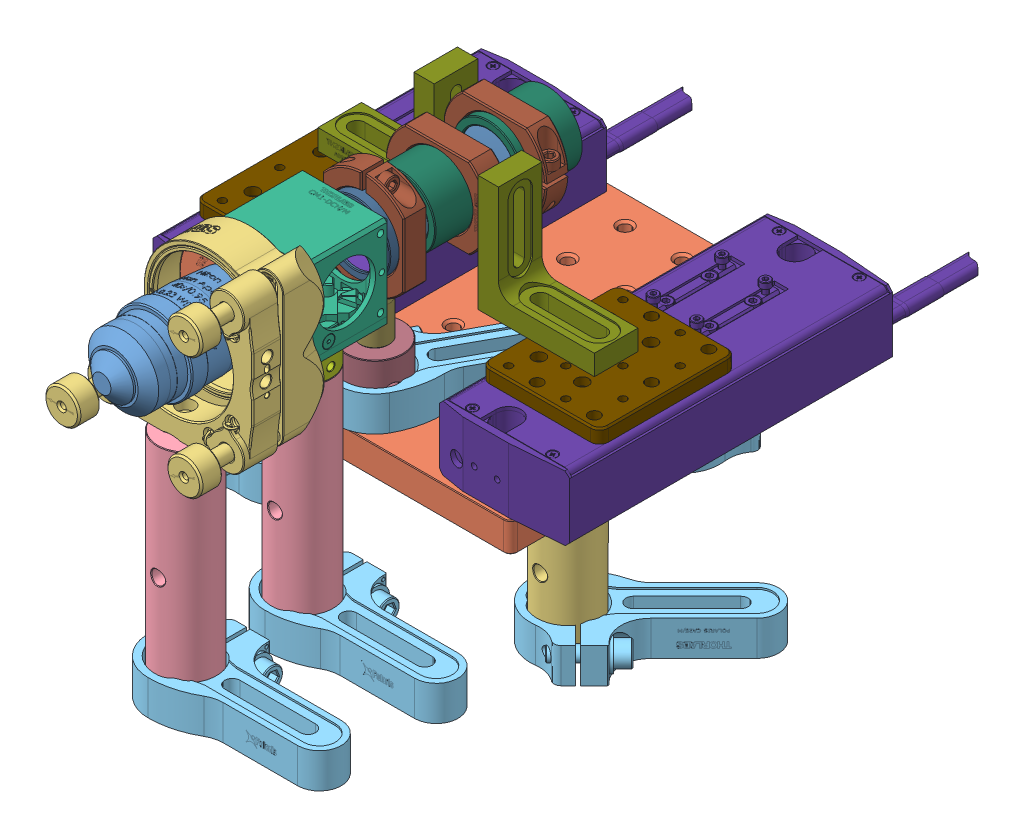
SolidWorks assembly Zoom_132.5-150mm, configuration Default. Lengths in mm.
Overall size (255.21 170.85 306.23).
40 component instances, 21 part files, 93 mates.
Components (placement in the parent):
- CFI Plan Apo Lambda 40x - 0.95NA, WD0.25-0.17, MRD00405-1: CFI Plan Apo Lambda 40x - 0.95NA, WD0.25-0.17, MRD00405 [Default] at origin size (34.5 34.5 64.68)
- SM2A33-Solidworks-1: SM2A33-Solidworks [Default] at (0 0 -62.1692) size (51.69 51.69 4.98)
- POLARIS-K2T-Solidworks-1: POLARIS-K2T-Solidworks [Default] at (40.1333 -35.7609 -82.8706) x (0 1 0) z (0 0 1) size (70.19 70.19 56.2)
- RS100_M-Solidworks-2: RS100_M-Solidworks [Default] at (2.2631 -83.8822 -39.0526) size (25 100 25.2)
- POLARIS-CA25_M-Solidworks-6: POLARIS-CA25_M-Solidworks [Default] at (53.6685 -156.438 -36.5961) size (84.45 15.24 40.64)
- CM1-DCH_M-Solidworks-1: CM1-DCH_M-Solidworks [Web Assembly] at (0 0 -87.73) size (38.1 45.72 38.1)
- RS9_M-Solidworks-1: RS9_M-Solidworks [Default] at (0 -31.17 -87.73) size (24.99 9 24.99)
- RS100_M-Solidworks-1: RS100_M-Solidworks [Default] at (2.2631 -83.9922 -90.0642) size (25 100 25.2)
- POLARIS-CA25_M-Solidworks-5: POLARIS-CA25_M-Solidworks [Default] at (53.6685 -156.438 -87.6077) size (84.45 15.24 40.64)
- 47649_25x300mm_achromat-1: 47649_25x300mm_achromat [Default] at (0 0 -111.23) x (-1 0 0) z (0 0 -1) size (25.49 25.5 5.5)
- SM1S1M-Solidworks-1: SM1S1M-Solidworks [Default] at (0.6703 -0.4225 -118.2048) x (1 0 0) z (0 -1 0) size (25.4 1 25.4)
- 47649_25x300mm_achromat-3: 47649_25x300mm_achromat [Default] at (0 0 -117.2046) x (-1 0 0) z (0 0 -1) size (25.49 25.5 5.5)
- SM1L05E-Solidworks-1: SM1L05E-Solidworks [Default] at (0 0 -124.3159) x (-0.994851 0.101347 0) z (0 0 -1) size (30.48 30.48 13.72)
- SM1RC_M-Solidworks-1: SM1RC_M-Solidworks [Web Drawing] at (0 0 -124.3159) size (35.56 44.69 10.16)
- TR20_M-Solidworks-1: TR20_M-Solidworks [Default] at (0 -42.0878 -119.2359) size (12.67 25.01 12.87)
- RS25_M-Solidworks-1: RS25_M-Solidworks [Default] at (0.0594 -54.2232 -117.8156) x (0.283723 0 -0.958906) z (0.958906 0 0.283723) size (25 25 25.2)
- POLARIS-CA25_M-Solidworks-1: POLARIS-CA25_M-Solidworks [Default] at (25.9778 -86.9658 -166.1985) x (0.482043 0 -0.876147) z (0.876147 0 0.482043) size (84.45 15.24 40.64)
- 62495_25xN150mm_achromat-1: 62495_25xN150mm_achromat [Default] at (0 0 -138.3146) size (25.81 25.77 8.99)
- SM1L10E-Solidworks-2: SM1L10E-Solidworks [Default] at (0 0 -156.7898) x (-1 0 0) z (0 0 -1) size (30.48 30.48 26.42)
- SM1RC_M-Solidworks-2: SM1RC_M-Solidworks [Web Drawing] at (0 0 -156.5528) x (0 1 0) z (0 0 1) size (35.56 44.69 10.16)
- AB90G-Solidworks-2: AB90G-Solidworks [Default] at (47.498 -6.6878 -151.8604) x (0 0 -1) z (1 0 0) size (19.05 50.8 50.8)
- DDS050_M-Solidworks-2: DDS050_M-Solidworks [Default] at (62.5 -67.0878 -177.7259) x (0 0 -1) z (1 0 0) size (194.32 35 57)
  - DDS050_M-Solidworks_base-1: DDS050_M-Solidworks_base [Default] at origin size (194.32 34 57)
  - DDS050_M-Solidworks_slider-1: DDS050_M-Solidworks_slider [Default] at (-50 0 0) size (60 6.2 52)
- 47647_25x250mm_achromat-1: 47647_25x250mm_achromat [Default] at (0 0 -169.0356) x (-1 0 0) z (0 0 -1) size (25.55 25.5 7.5)
- SM1S1M-Solidworks-2: SM1S1M-Solidworks [Default] at (0.6703 -0.4225 -177.9547) x (1 0 0) z (0 -1 0) size (25.4 1 25.4)
- 47647_25x250mm_achromat-2: 47647_25x250mm_achromat [Default] at (0 0 -176.9056) x (-1 0 0) z (0 0 -1) size (25.55 25.5 7.5)
- SM1L10E-Solidworks-1: SM1L10E-Solidworks [Default] at (0 0 -194.9224) x (-0.655081 -0.755559 0) z (0 0 -1) size (30.48 30.48 26.42)
- SM1RC_M-Solidworks-3: SM1RC_M-Solidworks [Web Drawing] at (0 0 -171.3928) x (0 1 0) z (0 0 -1) size (35.56 44.69 10.16)
- AB90G-Solidworks-1: AB90G-Solidworks [Default] at (-47.498 -6.6878 -176.8604) x (0 0 1) z (-1 0 0) size (19.05 50.8 50.8)
- DDS050_M-Solidworks-3: DDS050_M-Solidworks [Default] at (-62.5 -67.0878 -177.7259) x (0 0 -1) z (1 0 0) size (194.32 35 57)
  - DDS050_M-Solidworks_base-1: DDS050_M-Solidworks_base [Default] at origin size (194.32 34 57)
  - DDS050_M-Solidworks_slider-1: DDS050_M-Solidworks_slider [Default] at (-50 0 0) size (60 6.2 52)
- MB1515_M-Solidworks-2: MB1515_M-Solidworks [Default] at (0 -79.7878 -178.6259) size (150 12.7 150)
- RS50_M-Solidworks-1: RS50_M-Solidworks [Default] at (62.503 -106.6959 -139.8269) size (25 50 25.2)
- RS50_M-Solidworks-2: RS50_M-Solidworks [Default] at (-61.5441 -106.6959 -140.2463) x (0.678804 0 -0.734319) z (0.734319 0 0.678804) size (25 50 25.2)
- RS50_M-Solidworks-3: RS50_M-Solidworks [Default] at (13.7205 -106.6959 -240.681) x (0.344621 0 -0.938742) z (0.938742 0 0.344621) size (25 50 25.2)
- POLARIS-CA25_M-Solidworks-2: POLARIS-CA25_M-Solidworks [Default] at (100.3629 -101.442 -179.1618) x (0.707107 0 -0.707107) z (-0.707107 0 -0.707107) size (84.45 15.24 40.64)
- POLARIS-CA25_M-Solidworks-3: POLARIS-CA25_M-Solidworks [Default] at (-100.3629 -156.438 -179.1618) x (-0.707107 0 -0.707107) z (0.707107 0 -0.707107) size (84.45 15.24 40.64)
- POLARIS-CA25_M-Solidworks-4: POLARIS-CA25_M-Solidworks [Default] at (-25.5359 -101.442 -278.9888) x (-0.707107 0 -0.707107) z (-0.707107 0 0.707107) size (84.45 15.24 40.64)
Mates (geometry in assembly coordinates):
- Coincident1: coordinate: point of CFI Plan Apo Lambda 40x - 0.95NA, WD0.25-0.17, MRD00405-1; point of assembly
- Coincident3: coincident anti-aligned: line of 47649_25x300mm_achromat-1 through (0 0 -109.7924) axis (0 0 -1); line of assembly
- Coincident4: coincident aligned: plane of 47649_25x300mm_achromat-1 through (0 0 -111.23) normal (0 0 -1); plane of assembly through (0 0 -111.23) normal (0 0 -1)
- Coincident5: coincident aligned: plane of 47649_25x300mm_achromat-1; plane of assembly through (0 0 0) normal (0 1 0)
- Coincident6: coincident aligned: plane of CFI Plan Apo Lambda 40x - 0.95NA, WD0.25-0.17, MRD00405-1 through (0 0 0) normal (0 1 0); plane of assembly through (0 0 0) normal (0 1 0)
- Concentric54: concentric aligned: cylinder of CFI Plan Apo Lambda 40x - 0.95NA, WD0.25-0.17, MRD00405-1 through (0 0 0) axis (0 0 1) radius 11.9; cylinder of SM2A33-Solidworks-1 through (0 0 -53.151) axis (0 0 1) radius 12.5
- Coincident130: coincident anti-aligned: plane of CFI Plan Apo Lambda 40x - 0.95NA, WD0.25-0.17, MRD00405-1 through (0 13.5 -59.68) normal (0 0 -1); plane of SM2A33-Solidworks-1 through (0 25.4046 -59.68) normal (0 0 1)
- Concentric55: concentric aligned: cylinder of SM2A33-Solidworks-1 through (0 0 -53.151) axis (0 0 1) radius 25.8445; cylinder of POLARIS-K2T-Solidworks-1 through (0 0 -64.6584) axis (0 0 1) radius 25.8445
- Coincident131: coincident aligned: plane of SM2A33-Solidworks-1 through (0 25.4046 -64.6584) normal (0 0 -1); plane of POLARIS-K2T-Solidworks-1 through (-31.144 -14.6486 -64.6584) normal (0 0 -1)
- Parallel31: parallel anti-aligned: plane of POLARIS-K2T-Solidworks-1 through (0 -35.56 -27.8284) normal (0 -1 0); plane of assembly through (0 0 0) normal (0 1 0)
- Concentric56: concentric aligned: cylinder of POLARIS-K2T-Solidworks-1 through (0 -35.56 -36.7184) axis (0 -1 0) radius 2.3495; cylinder of RS100_M-Solidworks-2 through (0 -35.56 -36.7184) axis (0 -1 0) radius 12.5
- Coincident134: coincident anti-aligned: plane of POLARIS-K2T-Solidworks-1 through (0 -35.56 -27.8284) normal (0 -1 0); plane of RS100_M-Solidworks-2 through (0 -35.56 -36.7184) normal (0 1 0)
- Concentric57: concentric aligned: cylinder of RS100_M-Solidworks-2 through (0 -35.56 -36.7184) axis (0 -1 0) radius 12.5; cylinder of POLARIS-CA25_M-Solidworks-6 through (0 -121.32 -36.7184) axis (0 -1 0) radius 13.4938
- Distance6: distance = 1 mm aligned: plane of POLARIS-CA25_M-Solidworks-6 through (0 -136.56 -36.7184) normal (0 -1 0); plane of RS100_M-Solidworks-2 through (0 -135.56 -36.7184) normal (0 -1 0)
- Parallel32: parallel aligned: plane of POLARIS-K2T-Solidworks-1 through (7.6697 -7.2047 -30.3684) normal (0 0 1); plane of POLARIS-CA25_M-Solidworks-6 through (58.42 -121.32 -27.1934) normal (0 0 1)
- Concentric58: concentric anti-aligned: cylinder of CM1-DCH_M-Solidworks-1 through (0 0 -106.78) axis (0 0 -1) radius 12.8524; line of assembly
- Parallel33: parallel aligned: plane of CM1-DCH_M-Solidworks-1 through (-19.05 19.05 -68.68) normal (0 1 0); plane of assembly through (0 0 0) normal (0 1 0)
- Distance7: distance = 4 mm anti-aligned: plane of CFI Plan Apo Lambda 40x - 0.95NA, WD0.25-0.17, MRD00405-1 through (0 11.9 -64.68) normal (0 0 -1); plane of CM1-DCH_M-Solidworks-1 through (-19.05 -19.05 -68.68) normal (0 0 1)
- Concentric59: concentric aligned: cylinder of CM1-DCH_M-Solidworks-1 through (0 -26.67 -87.73) axis (0 -1 0) radius 2; cylinder of RS9_M-Solidworks-1 through (0 -26.67 -87.73) axis (0 -1 0) radius 12.4968
- Coincident139: coincident anti-aligned: plane of CM1-DCH_M-Solidworks-1 through (0 -26.67 -87.73) normal (0 -1 0); plane of RS9_M-Solidworks-1 through (0 -26.67 -87.73) normal (0 1 0)
- Concentric60: concentric aligned: cylinder of RS9_M-Solidworks-1 through (0 -26.67 -87.73) axis (0 -1 0) radius 12.4968; cylinder of RS100_M-Solidworks-1 through (0 -35.67 -87.73) axis (0 -1 0) radius 12.5
- Coincident140: coincident anti-aligned: plane of RS9_M-Solidworks-1 through (0 -35.67 -87.73) normal (0 -1 0); plane of RS100_M-Solidworks-1 through (0 -35.67 -87.73) normal (0 1 0)
- Concentric61: concentric aligned: cylinder of RS100_M-Solidworks-1 through (0 -35.67 -87.73) axis (0 -1 0) radius 12.5; cylinder of POLARIS-CA25_M-Solidworks-5 through (0 -121.32 -87.73) axis (0 -1 0) radius 13.4938
- Coincident141: coincident aligned: plane of POLARIS-CA25_M-Solidworks-6 through (0 -136.56 -36.7184) normal (0 -1 0); plane of POLARIS-CA25_M-Solidworks-5 through (0 -136.56 -87.73) normal (0 -1 0)
- Parallel34: parallel aligned: plane of POLARIS-CA25_M-Solidworks-6 through (58.42 -121.32 -27.1934) normal (0 0 1); plane of POLARIS-CA25_M-Solidworks-5 through (58.42 -121.32 -78.205) normal (0 0 1)
- Concentric62: concentric anti-aligned: cylinder of SM1S1M-Solidworks-1 through (0 0 -116.5623) axis (0 0 -1) radius 11.4935; line of assembly
- Tangent41: tangent: face of 47649_25x300mm_achromat-1; circle of SM1S1M-Solidworks-1
- Coincident143: coincident anti-aligned: line of 47649_25x300mm_achromat-3 through (0 0 -115.767) axis (0 0 -1); line of assembly
- Coincident144: coincident aligned: plane of 47649_25x300mm_achromat-3; plane of assembly through (0 0 0) normal (0 1 0)
- Tangent42: tangent: circle of SM1S1M-Solidworks-1; face of 47649_25x300mm_achromat-3
- Concentric63: concentric anti-aligned: cylinder of SM1L05E-Solidworks-1 through (0 0 -163.3362) axis (0 0 -1) radius 13.1445; line of assembly
- Tangent45: tangent: face of 47649_25x300mm_achromat-1; circle of SM1L05E-Solidworks-1
- Coincident146: coincident aligned: plane of SM1L05E-Solidworks-1 through (1.3322 13.0768 -124.3159) normal (0 0 -1); plane of SM1RC_M-Solidworks-1 through (0 0 -124.3159) normal (0 0 -1)
- Concentric64: concentric anti-aligned: cylinder of SM1L05E-Solidworks-1 through (0 0 -163.3362) axis (0 0 -1) radius 15.24; cylinder of SM1RC_M-Solidworks-1 through (0 0 -124.3159) axis (0 0 1) radius 15.3035
- Parallel36: parallel anti-aligned: plane of SM1RC_M-Solidworks-1 through (0 -22.098 -124.3159) normal (0 -1 0); plane of assembly through (0 0 0) normal (0 1 0)
- Concentric65: concentric aligned: cylinder of SM1RC_M-Solidworks-1 through (0 -22.098 -119.2359) axis (0 -1 0) radius 2; cylinder of TR20_M-Solidworks-1 through (0 -29.145 -119.2359) axis (0 -1 0) radius 2
- Coincident149: coincident anti-aligned: plane of SM1RC_M-Solidworks-1 through (0 -22.098 -124.3159) normal (0 -1 0); plane of TR20_M-Solidworks-1 through (0 -22.098 -119.2359) normal (0 1 0)
- Concentric66: concentric anti-aligned: cylinder of TR20_M-Solidworks-1 through (0 -22.098 -119.2359) axis (0 1 0) radius 6.3373; cylinder of RS25_M-Solidworks-1 through (0 -42.0878 -119.2359) axis (0 -1 0) radius 12.5
- Coincident150: coincident anti-aligned: plane of TR20_M-Solidworks-1 through (5.8293 -42.0878 -119.2359) normal (0 -1 0); plane of RS25_M-Solidworks-1 through (0 -42.0878 -119.2359) normal (0 1 0)
- Concentric67: concentric aligned: cylinder of RS25_M-Solidworks-1 through (0 -42.0878 -119.2359) axis (0 -1 0) radius 12.5; cylinder of POLARIS-CA25_M-Solidworks-1 through (0 -51.8478 -119.2359) axis (0 -1 0) radius 13.4938
- Coincident151: coincident aligned: plane of RS25_M-Solidworks-1 through (0 -67.0878 -119.2359) normal (0 -1 0); plane of POLARIS-CA25_M-Solidworks-1 through (0 -67.0878 -119.2359) normal (0 -1 0)
- Distance10: distance = 9.05 mm anti-aligned: plane of 47649_25x300mm_achromat-3 through (0 0 -122.7046) normal (0 0 -1); plane of 62495_25xN150mm_achromat-1 through (0 0 -131.7546) normal (0 0 1)
- Coincident154: coincident aligned: line of 62495_25xN150mm_achromat-1 through (0 0 -140.1587) axis (0 0 1); line of assembly
- Coincident155: coincident aligned: plane of 62495_25xN150mm_achromat-1 through (0 0 -138.3146) normal (0 1 0); plane of assembly through (0 0 0) normal (0 1 0)
- Concentric68: concentric anti-aligned: cylinder of SM1L10E-Solidworks-2 through (0 0 -195.81) axis (0 0 -1) radius 13.1445; line of assembly
- Coincident156: coincident anti-aligned: plane of 62495_25xN150mm_achromat-1 through (0 0 -131.3898) normal (0 0 1); plane of SM1L10E-Solidworks-2 through (0 13.1445 -131.3898) normal (0 0 -1)
- Distance11: distance = 0.237 mm aligned: plane of SM1RC_M-Solidworks-2 through (0 0 -156.5528) normal (0 0 -1); plane of SM1L10E-Solidworks-2 through (0 13.1445 -156.7898) normal (0 0 -1)
- Concentric69: concentric anti-aligned: cylinder of SM1L10E-Solidworks-2 through (0 0 -195.81) axis (0 0 -1) radius 15.24; cylinder of SM1RC_M-Solidworks-2 through (0 0 -156.5528) axis (0 0 1) radius 15.3035
- Parallel37: parallel aligned: plane of SM1RC_M-Solidworks-2 through (0 17.78 -156.5528) normal (0 1 0); plane of assembly through (0 0 0) normal (0 1 0)
- Tangent47: tangent anti-aligned: cylinder of SM1RC_M-Solidworks-2 through (22.098 0 -151.4728) axis (1 0 0) radius 2; plane of AB90G-Solidworks-2 through (22.098 11.0922 -149.4728) normal (0 0 -1)
- Distance12: distance = 0.9322 mm aligned: plane of AB90G-Solidworks-2 through (30.988 18.7122 -161.3854) normal (0 1 0); plane of SM1RC_M-Solidworks-2 through (0 17.78 -156.5528) normal (0 1 0)
- Coincident162: coincident anti-aligned: plane of SM1RC_M-Solidworks-2 through (22.098 0 -156.5528) normal (1 0 0); plane of AB90G-Solidworks-2 through (22.098 18.7122 -161.3854) normal (-1 0 0)
- Coincident163: coincident anti-aligned: plane of AB90G-Solidworks-2 through (22.098 -32.0878 -161.3854) normal (0 -1 0); plane of DDS050_M-Solidworks-2/DDS050_M-Solidworks_slider-1 through (42.748 -32.0878 -182.7259) normal (0 1 0)
- Distance13: distance = 21.85 mm aligned: plane of AB90G-Solidworks-2 through (72.898 -32.0878 -161.3854) normal (1 0 0); plane of DDS050_M-Solidworks-2/DDS050_M-Solidworks_slider-1 through (94.748 -32.0878 -122.7259) normal (1 0 0)
- Tangent48: tangent anti-aligned: plane of AB90G-Solidworks-2 through (47.498 -32.0878 -155.2259) normal (0 0 1); cylinder of DDS050_M-Solidworks-2/DDS050_M-Solidworks_slider-1 through (62.498 -32.0878 -152.7259) axis (0 1 0) radius 2.5
- Tangent49: tangent anti-aligned: plane of AB90G-Solidworks-2 through (47.498 -32.0878 -155.2259) normal (0 0 1); cylinder of DDS050_M-Solidworks-2/DDS050_M-Solidworks_slider-1 through (62.498 -32.0878 -152.7259) axis (0 1 0) radius 2.5
- Distance14: distance = 30.721 mm anti-aligned: plane of 62495_25xN150mm_achromat-1 through (0 0 -138.3146) normal (0 0 1); plane of 47647_25x250mm_achromat-1 through (0 0 -169.0356) normal (0 0 -1)
- Coincident166: coincident anti-aligned: line of 47647_25x250mm_achromat-1 through (0 0 -167.6746) axis (0 0 -1); line of assembly
- Coincident167: coincident aligned: plane of 47647_25x250mm_achromat-1; plane of assembly through (0 0 0) normal (0 1 0)
- Concentric70: concentric anti-aligned: cylinder of SM1S1M-Solidworks-2 through (0 0 -176.3122) axis (0 0 -1) radius 11.4935; line of assembly
- Tangent50: tangent: face of 47647_25x250mm_achromat-1; circle of SM1S1M-Solidworks-2
- Coincident168: coincident anti-aligned: line of 47647_25x250mm_achromat-2 through (0 0 -175.5446) axis (0 0 -1); line of assembly
- Distance15: distance = 0.37 mm aligned: plane of 47647_25x250mm_achromat-1 through (0 0 -176.5356) normal (0 0 -1); plane of 47647_25x250mm_achromat-2 through (0 0 -176.9056) normal (0 0 -1)
- Coincident170: coincident aligned: plane of 47647_25x250mm_achromat-2; plane of assembly through (0 0 0) normal (0 1 0)
- Concentric73: concentric anti-aligned: cylinder of SM1L10E-Solidworks-1 through (0 0 -233.9427) axis (0 0 -1) radius 15.24; line of assembly
- Coincident171: coincident aligned: circle of 47647_25x250mm_achromat-1; plane of SM1L10E-Solidworks-1 through (-9.9314 8.6107 -169.5224) normal (0 0 -1)
- Distance16: distance = 2.8864 mm aligned: plane of SM1RC_M-Solidworks-3 through (0 0 -171.3928) normal (0 0 1); plane of SM1L10E-Solidworks-1 through (-11.5147 9.9834 -168.5064) normal (0 0 1)
- Concentric74: concentric aligned: cylinder of SM1L10E-Solidworks-1 through (0 0 -233.9427) axis (0 0 -1) radius 15.24; cylinder of SM1RC_M-Solidworks-3 through (0 0 -171.3928) axis (0 0 -1) radius 15.3035
- Parallel38: parallel aligned: plane of SM1RC_M-Solidworks-3 through (0 17.78 -171.3928) normal (0 1 0); plane of assembly through (0 0 0) normal (0 1 0)
- Tangent62: tangent anti-aligned: cylinder of SM1RC_M-Solidworks-3 through (-22.098 0 -176.4728) axis (-1 0 0) radius 2; plane of AB90G-Solidworks-1 through (-22.098 11.0922 -174.4728) normal (0 0 -1)
- Distance17: distance = 0.9322 mm aligned: plane of AB90G-Solidworks-1 through (-30.988 18.7122 -167.3354) normal (0 1 0); plane of SM1RC_M-Solidworks-3 through (0 17.78 -171.3928) normal (0 1 0)
- Coincident175: coincident anti-aligned: plane of SM1RC_M-Solidworks-3 through (-22.098 0 -171.3928) normal (-1 0 0); plane of AB90G-Solidworks-1 through (-22.098 18.7122 -167.3354) normal (1 0 0)
- Coincident176: coincident anti-aligned: plane of AB90G-Solidworks-1 through (-22.098 -32.0878 -167.3354) normal (0 -1 0); plane of DDS050_M-Solidworks-3/DDS050_M-Solidworks_slider-1 through (-82.252 -32.0878 -182.7259) normal (0 1 0)
- Distance18: distance = 9.354 mm aligned: plane of AB90G-Solidworks-1 through (-72.898 -32.0878 -167.3354) normal (-1 0 0); plane of DDS050_M-Solidworks-3/DDS050_M-Solidworks_slider-1 through (-82.252 -32.0878 -122.7259) normal (-1 0 0)
- Tangent63: tangent anti-aligned: plane of AB90G-Solidworks-1 through (-47.498 -32.0878 -180.2259) normal (0 0 1); cylinder of DDS050_M-Solidworks-3/DDS050_M-Solidworks_slider-1 through (-62.502 -32.0878 -177.7259) axis (0 1 0) radius 2.5
- Coincident178: coincident aligned: plane of MB1515_M-Solidworks-2 through (0 -79.7878 -178.6259) normal (1 0 0); plane of assembly through (0 0 0) normal (1 0 0)
- Coincident179: coincident anti-aligned: plane of DDS050_M-Solidworks-3/DDS050_M-Solidworks_base-1 through (-62.5 -67.0878 -177.7259) normal (0 -1 0); plane of MB1515_M-Solidworks-2 through (-72 -67.0878 -106.6259) normal (0 1 0)
- Tangent65: tangent aligned: cylinder of DDS050_M-Solidworks-3/DDS050_M-Solidworks_base-1 through (-62.5 -40.3878 -115.2259) axis (0 1 0) radius 3.4; cylinder of MB1515_M-Solidworks-2 through (-62.5 -67.0878 -116.1259) axis (0 1 0) radius 2.5
- Concentric77: concentric anti-aligned: cylinder of MB1515_M-Solidworks-2 through (62.5 -67.0878 -141.1259) axis (0 1 0) radius 2.5; cylinder of RS50_M-Solidworks-1 through (62.5 -79.7878 -141.1259) axis (0 -1 0) radius 12.5
- Coincident180: coincident anti-aligned: plane of MB1515_M-Solidworks-2 through (-72 -79.7878 -106.6259) normal (0 -1 0); plane of RS50_M-Solidworks-1 through (62.5 -79.7878 -141.1259) normal (0 1 0)
- Concentric78: concentric anti-aligned: cylinder of MB1515_M-Solidworks-2 through (-62.5 -67.0878 -141.1259) axis (0 1 0) radius 2.5; cylinder of RS50_M-Solidworks-2 through (-62.5 -79.7878 -141.1259) axis (0 -1 0) radius 12.5
- Coincident181: coincident anti-aligned: plane of MB1515_M-Solidworks-2 through (-72 -79.7878 -106.6259) normal (0 -1 0); plane of RS50_M-Solidworks-2 through (-62.5 -79.7878 -141.1259) normal (0 1 0)
- Concentric79: concentric anti-aligned: cylinder of MB1515_M-Solidworks-2 through (12.5 -67.0878 -241.1259) axis (0 1 0) radius 2.5; cylinder of RS50_M-Solidworks-3 through (12.5 -79.7878 -241.1259) axis (0 -1 0) radius 12.5
- Coincident182: coincident anti-aligned: plane of MB1515_M-Solidworks-2 through (-72 -79.7878 -106.6259) normal (0 -1 0); plane of RS50_M-Solidworks-3 through (12.5 -79.7878 -241.1259) normal (0 1 0)
- Concentric80: concentric anti-aligned: cylinder of RS50_M-Solidworks-1 through (62.5 -79.7878 -141.1259) axis (0 -1 0) radius 12.5; cylinder of POLARIS-CA25_M-Solidworks-2 through (62.5 -136.56 -141.1259) axis (0 1 0) radius 13.4938
- Coincident183: coincident aligned: plane of POLARIS-CA25_M-Solidworks-6 through (0 -136.56 -36.7184) normal (0 -1 0); plane of POLARIS-CA25_M-Solidworks-2 through (62.5 -136.56 -141.1259) normal (0 -1 0)
- Angle1: planar angle = 0.785398 rad aligned: plane of POLARIS-CA25_M-Solidworks-2 through (110.5444 -136.56 -175.6999) normal (0.707107 0 0.707107); plane of MB1515_M-Solidworks-2 through (75 -67.0878 -106.6259) normal (1 0 0)
- Concentric81: concentric aligned: cylinder of RS50_M-Solidworks-2 through (-62.5 -79.7878 -141.1259) axis (0 -1 0) radius 12.5; cylinder of POLARIS-CA25_M-Solidworks-3 through (-62.5 -121.32 -141.1259) axis (0 -1 0) radius 13.4938
- Coincident185: coincident aligned: plane of POLARIS-CA25_M-Solidworks-6 through (0 -136.56 -36.7184) normal (0 -1 0); plane of POLARIS-CA25_M-Solidworks-3 through (-62.5 -136.56 -141.1259) normal (0 -1 0)
- Angle2: planar angle = 0.785398 rad aligned: plane of POLARIS-CA25_M-Solidworks-3 through (-110.5444 -121.32 -175.6999) normal (-0.707107 0 0.707107); plane of MB1515_M-Solidworks-2 through (-75 -67.0878 -106.6259) normal (-1 0 0)
- Coincident187: coincident aligned: plane of POLARIS-CA25_M-Solidworks-2 through (62.5 -136.56 -141.1259) normal (0 -1 0); plane of POLARIS-CA25_M-Solidworks-4 through (12.5 -136.56 -241.1259) normal (0 -1 0)
- Concentric82: concentric anti-aligned: cylinder of RS50_M-Solidworks-3 through (12.5 -79.7878 -241.1259) axis (0 -1 0) radius 12.5; cylinder of POLARIS-CA25_M-Solidworks-4 through (12.5 -136.56 -241.1259) axis (0 1 0) radius 13.4938
- Angle3: planar angle = 0.785398 rad aligned: plane of POLARIS-CA25_M-Solidworks-4 through (-22.074 -136.56 -289.1703) normal (0.707107 0 -0.707107); plane of MB1515_M-Solidworks-2 through (-72 -67.0878 -253.6259) normal (0 0 -1)
